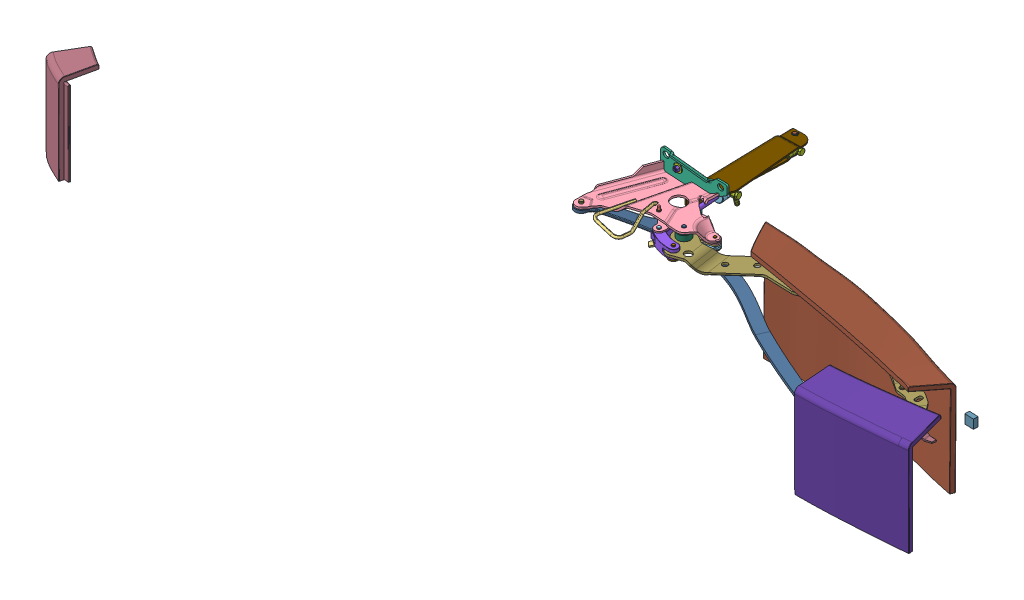
SolidWorks assembly 1 - TOIT ESCAMOTABLE, configuration Défaut. Lengths in mm.
Overall size (1763.8 334.82 831.05).
65 component instances, 51 part files, 23 mates.
Components (placement in the parent):
- Biellette 4-1: Biellette 4 [Défaut] at (-1551.2521 -414.2318 1656.9047) x (0.468484 -0.000409 -0.883472) z (0.883472 0.000057 0.468484) size (112.69 33.11 82.41)
  - 4-1: 4 [Défaut] at (2225.7827 591.5208 703.2597) x (0.218461 0.000145 -0.975846) z (0.975846 0.000386 0.218461) size (18 8 18)
  - 46-1: 46 [Défaut] at origin size (29.25 21.01 36.3)
  - 50_2-1: 50_2 [Défaut] at origin size (111.95 25.05 78.84)
  - 50_1-1: 50_1 [Défaut] at (0.2445 -0.873 -0.0377) x (1 0.00041 0.000002) z (-0.000002 -0.000057 1) size (102 23.39 81.66)
  - 52BIS-1: 52BIS [Défaut] at (1803.6304 -3.2417 -1581.4602) x (0.452996 0.000134 0.891513) z (-0.891513 -0.00039 0.452996) size (20 32 20)
- Biellette 5-1: Biellette 5 [Défaut] at (-1783.7087 -415.1645 1380.9797) x (0.603911 0 -0.797052) z (0.797052 0 0.603911) size (40.38 26.6 70.86)
  - 47-1: 47 [Défaut] at (0.0788 -0.3457 -0.1198) x (1 0.000129 0) z (0 -0.000197 1) size (10 4 10)
  - 48-1: 48 [Défaut] at (0.0788 0.0408 -0.1198) x (1 0.000129 0) z (0 -0.000197 1) size (10 4 10)
  - 51-1: 51 [Défaut] at origin size (36.66 20.6 67.14)
  - 52-1: 52 [Défaut] at (-61.137 -0.0001 1211.0461) x (0.858083 0 -0.513511) z (0.513511 0 0.858083) size (20 26.6 20)
- Bras d'articulation 8-1: Bras d'articulation 8 [Défaut] at (1109.5772 -414.3873 1924.2232) x (-0.822194 -0.000049 -0.569208) z (0.569208 -0.000113 -0.822194) size (513.66 101.01 316.13)
  - 27-1: 27 [Défaut] at origin size (513.66 100.48 316.13)
  - 28-2: 28 [Défaut] at (0.0061 -0.1899 0.0459) x (1 0.000049 0) z (0 0.000113 1) size (20 8 20)
  - 29-1: 29 [Défaut] at (-485.0397 -93.1918 287.2564) x (1 0.000049 0) z (0 0.000113 1) size (20 8 20)
- Pavillon 7-1: Pavillon 7 [Défaut] at (-973.4618 -416.6967 -1067.8554) x (0.99643 0.000086 0.084422) z (-0.084422 0.001929 0.996428) size (317.83 232 129.49)
  - 44-1: 44 [Défaut] at origin size (219.19 23.25 101.49)
  - 1615-1: 1615 [Défaut] at (-0.9791 4.8613 -2.1044) x (1 -0.00011 -0.000288) z (0.000288 -0.004457 0.99999) size (98.08 52.67 74.97)
  - Hex Flange Bolt Small_ISO-2: Hex Flange Bolt Small_ISO [ISO 4162 - M6 x 12 x 12-N] at (1589.2084 535.554 1078.7736) x (0.064417 -0.997916 -0.003841) z (0.639494 0.038325 0.76784) size (18.8 13.6 13.6)
  - Hex Flange Bolt Small_ISO-3: Hex Flange Bolt Small_ISO [ISO 4162 - M6 x 12 x 12-N] at (1635.0058 538.5525 1067.8078) x (0.064417 -0.997916 -0.003841) z (0.639494 0.038325 0.76784) size (18.8 13.6 13.6)
  - 40-2: 40 [Défaut] at (3505.3536 1063.4304 1051.0405) x (-0.841704 0.012388 -0.539798) z (-0.539827 -0.039772 0.840836) size (13.37 5.84 13.08)
  - 40-3: 40 [Défaut] at (3551.1511 1066.4289 1040.0747) x (-0.841704 0.012388 -0.539798) z (-0.539827 -0.039772 0.840836) size (13.37 5.84 13.08)
  - PAVILLON-1: PAVILLON [Défaut] at (1497.6236 449.6532 1038.2886) x (0.998995 -0.006358 -0.044377) z (-0.006846 -0.999918 -0.010851) size (312.04 111.12 228.8)
  - 34-1: 34 [Défaut] at (-0.1051 1.9936 -0.8757) x (1 -0.000013 0) z (0 -0.001928 0.999998) size (20 7 20)
  - 39_1-1: 39_1 [Défaut] at (1705.3024 528.4997 1021.2431) x (1 -0.000086 0) z (0 -0.001929 0.999998) size (20 16.5 20)
  - 43_1-1: 43_1 [Défaut] at (1538.1186 520.3687 1092.9033) x (-0.912008 0.00087 -0.410172) z (-0.410173 -0.001724 0.912006) size (20 17.5 20)
- Cylindre vérin 2-1: Cylindre vérin 2 [Défaut] at (-159.1778 138.3124 6.0203) x (0.545107 -0.837169 -0.044791) z (-0.834357 -0.546944 0.068558) size (66.63 202.27 72.2)
  - Vérin tube-1: Vérin tube [Défaut] at (67.1722 -78.4933 -191.3212) x (-0.401704 0 -0.915769) z (-0.915769 0 0.401704) size (23 150 23)
  - Vérin corps3-1: Vérin corps3 [Défaut] at (67.1722 -224.4933 -191.3212) x (-0.837169 0 -0.546944) z (-0.546944 0 0.837169) size (26 29 26)
  - Vérin corps1-1: Vérin corps1 [Défaut] at (67.1722 -82.4933 -191.3212) x (0.837169 0 0.546944) z (-0.546944 0 0.837169) size (27 29 27)
  - Vérin bague-1: Vérin bague [Défaut] at (68.2187 -244.6933 -190.6375) x (-0.537418 -0.185827 0.822588) z (-0.101637 0.982583 0.155568) size (16 11.5 16)
  - Vérin bague-2: Vérin bague [Défaut] at (66.1257 -244.6933 -192.0049) x (0.299148 0.837169 -0.457885) z (-0.457885 0.546944 0.700852) size (16 11.5 16)
  - vérin 1-1: vérin 1 [Défaut] at (-547.758 -937.2273 1850.5736) x (0.542849 0.122243 -0.830886) z (-0.066861 0.9925 0.102337) size (43.79 33.68 170.02)
- Tige vérin 3-1: Tige vérin 3 [Défaut] at (106.3732 186.72 -57.6246) x (0.996641 0 -0.081893) z (0 -1 0) size (20 221.5 20)
  - Vérin tige-1: Vérin tige [Défaut] at (-72.9634 -64.1363 0) size (20 221.5 20)
  - Vérin btige-1: Vérin btige [Défaut] at (-72.9634 128.3637 6) x (1 0 0) z (0 1 0) size (10 12 10)
- Lunette arrière 6-1: Lunette arrière 6 [Défaut] at (77.9117 193.67 53.9597) x (-0.919233 0 -0.393714) z (0.393714 0 -0.919233) size (583.86 314.32 496.34)
  - 37-1: 37 [Défaut] at origin size (18 11 18)
  - LUNETTE-1: LUNETTE [Défaut] at (-284.1034 -251.0618 157.7611) x (0.985549 -0.006556 0.169266) z (-0.004926 -0.999937 -0.010051) size (477.42 277.59 308.69)
  - 37-2: 37 [Défaut] at (0 -1 0) x (-0.72009 0 -0.693881) z (-0.693881 0 0.72009) size (18 11 18)
  - 32-1: 32 [Défaut] at (-2015.7981 -609.4617 -1136.448) x (0.982385 0.000417 0.18687) z (-0.186869 -0.00037 0.982385) size (527.96 70.41 348.72)
  - 36-1: 36 [Défaut] at (-2016.1005 -611.023 -1135.4876) x (0.982355 -0.000016 0.187027) z (-0.187027 0.001978 0.982353) size (36.02 26.21 44.06)
  - 35-1: 35 [Défaut] at (-2014.1899 -614.939 -1136.2657) x (0.982319 0.002577 0.187197) z (-0.187199 0.000642 0.982322) size (15.92 27.09 17.3)
  - 31-1: 31 [Défaut] at (-2015.7211 -609.9779 -1136.6628) x (0.982385 0.000464 0.18687) z (-0.186869 -0.000753 0.982384) size (28.01 19.02 28.01)
  - 30-1: 30 [Défaut] at (-2016.1086 -608.8253 -1136.2496) x (0.982385 0 0.18687) z (-0.18687 0 0.982385) size (18 7 18)
- Support 1-1: Support 1 [Défaut] at (-2066.3679 -416.0573 -816.6479) x (0.998169 0 0.060485) z (-0.060485 0 0.998169) size (1700.94 301.28 729.5)
  - Bati-1: Bati [Défaut] at origin size (229.41 180.55 405.54)
    - 8-1: 8 [Défaut] at (1.3849 0.8394 2.1491) x (0.999999 0 -0.001165) z (0.001165 0 0.999999) size (12 12 24)
    - 17-1: 17 [Défaut] at (-4.2516 0.8356 14.1603) x (0.99998 0.000022 -0.006399) z (0.006399 0.000071 0.99998) size (73.09 38.15 242.39)
    - 19-1: 19 [Défaut] at (-1.1151 0.8394 2.152) x (0.999999 0 -0.001165) z (0.001165 0 0.999999) size (67.06 96.47 36.71)
    - 20-1: 20 [Défaut] at (0.0666 1.2273 -0.7048) size (8 9 8)
    - 21-1: 21 [Défaut] at (-0.8363 1.2063 2.4626) x (0.999999 0 -0.001162) z (0.001162 0.000001 0.999999) size (68.39 27.16 100.85)
    - 22-1: 22 [Défaut] at (-0.7553 1.2 2.3791) x (0.999999 0.000003 -0.001165) z (0.001165 0 0.999999) size (228.74 37.96 169.9)
    - 25-1: 25 [Défaut] at (-0.7499 -0.7906 2.3623) x (0.999999 0 -0.001165) z (0.001165 0 0.999999) size (105.24 22.69 98.48)
    - 100s-1: 100s [Défaut] at (-1.1151 0.8394 2.152) x (0.999999 0 -0.001165) z (0.001165 0 0.999999) size (168.32 169.73 50.42)
    - Plain Washer Large Grade AC_ISO-1: Plain Washer Large Grade AC_ISO [Rondelle plate ISO 7093 - 6] at (2079.9412 636.9794 650.6657) x (-0.001165 0 -0.999999) z (0.923807 -0.382856 -0.001077) size (1.6 18 18)
    - Hex Nut GradeC_ISO-1: Hex Nut GradeC_ISO [Ecrou H ISO - 4034 - M6 - N] at (2079.9502 636.9794 658.3657) x (0.999999 0.000066 -0.001165) z (0.001165 0 0.999999) size (10 11.55 6.1)
  - 45-1: 45 [Défaut] at (2225.8504 606.2461 703.0279) x (0.307349 0 -0.951597) z (-0.951597 0 -0.307349) size (20 22.5 20)
  - 23-1: 23 [Défaut] at (2193.0126 626.2273 739.3162) x (-0.959508 0 -0.281682) z (-0.281682 0 0.959508) size (20 35.5 20)
  - Axe vérin-1: Axe vérin [Défaut] at (2117.3555 621.9041 434.2046) x (0 -1 0) z (-0.355439 0 -0.9347) size (38 8 8)
  - 26-1: 26 [Défaut] at (-100.5064 2.9741 322.5535) x (0.987978 -0.000721 -0.15459) z (0.15459 -0.000039 0.987979) size (20 19.51 20)
  - PARE BRISE-1: PARE BRISE [Défaut] at (1196.1951 453.584 992.7592) x (-0.006782 -0.999937 -0.008905) z (-0.986389 0.008152 -0.164224) size (201.63 92.79 80.23)
  - Butée coffre-1: Butée coffre [Défaut] at (2793.8268 591.5208 658.3345) x (0 -1 0) z (0.013055 0 0.999915) size (20 20 10)
  - anneauext6-1: anneauext6 [Défaut] at (2113.6167 585.9041 435.6264) x (0.433078 0 0.901357) z (0 -1 0) size (9.8 11.86 0.8)
  - anneauext6-2: anneauext6 [Défaut] at (2113.6167 620.7041 435.6264) x (0.433078 0 0.901357) z (0 -1 0) size (9.8 11.86 0.8)
Mates (geometry in assembly coordinates):
- Coaxial6: concentric aligned: cylinder of ?; cylinder of ?
- Distance12: distance = 0.25 mm anti-aligned: plane of ? through (-1551.171 197.42 1656.6713) normal (0 -1 0); plane of ? through (67.617 197.17 43.878) normal (0 1 0)
- Coaxial15: concentric aligned: cylinder of Cylindre vérin 2-1/Vérin corps1-1; cylinder of Tige vérin 3-1/Vérin tige-1
- Coaxial16: concentric anti-aligned: cylinder of ?; cylinder of Tige vérin 3-1/Vérin btige-1
- Distance11: distance = 0.4 mm anti-aligned: plane of ? through (-16.4711 193.12 49.7335) normal (0 -1 0); plane of Tige vérin 3-1/Vérin tige-1 through (35.9342 192.72 85.9899) normal (0 1 0)
- Coaxial25: concentric aligned: cylinder of Bras d'articulation 8-1/29-1; cylinder of Pavillon 7-1/43_1-1
- Coïncidente29: coincident anti-aligned: plane of Bras d'articulation 8-1/29-1 through (466.941 91.4115 149.9913) normal (0 -1 0); plane of Pavillon 7-1/43_1-1 through (461.1718 91.4115 146.7856) normal (0 1 0)
- Coaxial98: concentric anti-aligned: cylinder of Pavillon 7-1/39_1-1; cylinder of Lunette arrière 6-1/32-1
- Coaxial99: concentric anti-aligned: cylinder of ?; cylinder of Lunette arrière 6-1/30-1
- Coïncidente101: coincident anti-aligned: plane of ? through (76.1108 183.37 100.2215) normal (0 1 0); plane of Lunette arrière 6-1/30-1 through (91.8048 183.37 91.4695) normal (0 -1 0)
- Coïncidente149: coincident anti-aligned: plane of Bras d'articulation 8-1/28-2 through (-103.5628 192.422 104.3387) normal (0 1 0); plane of Support 1-1/Bati-1/22-1 through (-2067.2657 192.422 -814.3189) normal (0 -1 0)
- Coaxial136: concentric anti-aligned: cylinder of Biellette 4-1/4-1; cylinder of Support 1-1/Bati-1/25-1
- Coïncidente151: coincident anti-aligned: plane of Lunette arrière 6-1/37-1 through (71.661 204.67 51.2825) normal (0 1 0); plane of Support 1-1/Bati-1/22-1 through (184.9959 204.67 -74.1233) normal (0 -1 0)
- Coaxial137: concentric aligned: cylinder of Lunette arrière 6-1/37-2; cylinder of Support 1-1/Bati-1/25-1
- Coaxial140: concentric anti-aligned: cylinder of Cylindre vérin 2-1/Vérin bague-2; cylinder of Support 1-1/Bati-1/17-1
- Coaxial142: concentric anti-aligned: cylinder of Biellette 4-1/4-1; cylinder of Support 1-1/45-1
- Coaxial143: concentric aligned: cylinder of Lunette arrière 6-1/37-2; cylinder of Support 1-1/23-1
- Coaxial144: concentric aligned: cylinder of Bras d'articulation 8-1/28-2; cylinder of Support 1-1/26-1
- Coaxial145: concentric aligned: cylinder of Bras d'articulation 8-1/28-2; cylinder of Support 1-1/26-1
- TOIT INTER: planar angle = 0.15708 rad aligned: unknown of ?
- TOIT FERME: tangent anti-aligned: cylinder of ?; face of ?
- TOIT OUVERT: unknown = 4169.1578 mm aligned: unknown of ?; unknown of Support 1-1/Bati-1/22-1
- EFFORT MAXI: unknown = 1156.7195 mm anti-aligned: unknown of Lunette arrière 6-1/32-1; unknown of Support 1-1/Bati-1/22-1
